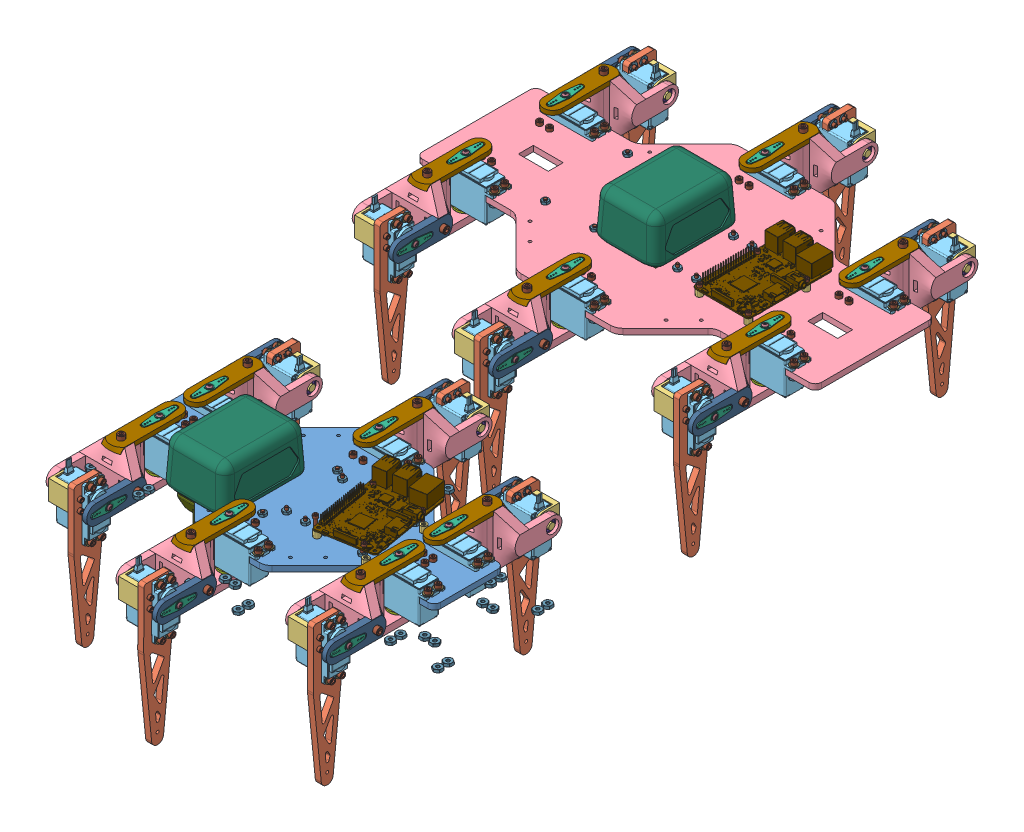
SolidWorks assembly Assem1, configuration Default. Lengths in mm. (continued)
Components (placement in the parent): (continued)
- Hexapod_NewBody-1: Hexapod_NewBody [Défaut] at origin size (371.2 181.88 349.28) (continued)
  - Battery-1: Battery [Défaut] at (-209.6397 14.6626 -46.247) x (-1 0 0) z (0 0 1) size (64.47 74.3 85.78) (continued)
    - MAKITA 4.0AH MOBILE-1: MAKITA 4.0AH MOBILE [Défaut] at (0.5853 -39.3124 91.7936) size (45.84 26.68 66.29)
  - arduinoMega-1: arduinoMega [Detailed] at (-189.11 -7.6 22.62) x (0 0 -1) z (-1 0 0) size (108.32 14.5 53.3)
  - raspberryPi3B-1: raspberryPi3B [Detailed] at (-100.6704 6.35 5.1405) x (-0.167042 0 -0.98595) z (0 1 0) size (87.05 58.5 19.5)
  - 12Channel PWM-1: 12Channel PWM [Default] at (-145.6 -5.6 15) x (-1 0 0) z (0 0 1) size (25.4 7.55 66.7)
  - DROK_090483.stp-1: DROK_090483.stp [Default] at (-77.5 -5.6 45) x (-1 0 0) z (0 -1 0) size (50.02 60 18.9)
  - socket head cap screw_ai-2: socket head cap screw_ai [HX-SHCS 0.138-32x0.625x0.625-N] at (-40.288 3.5052 19.09) x (0 -1 0) z (1 0 0) size (19.38 5.74 5.74)
  - socket head cap screw_ai-3: socket head cap screw_ai [HX-SHCS 0.138-32x0.625x0.625-N] at (-50.288 3.5052 19.09) x (0 -1 0) z (0.5 0 0.866025) size (19.38 5.74 5.74)
  - socket head cap screw_ai-4: socket head cap screw_ai [HX-SHCS 0.138-32x0.625x0.625-N] at (-50.288 3.5052 10.91) x (0 -1 0) z (1 0 0) size (19.38 5.74 5.74)
  - socket head cap screw_ai-5: socket head cap screw_ai [HX-SHCS 0.138-32x0.625x0.625-N] at (-40.288 3.5052 10.91) x (0 -1 0) z (1 0 0) size (19.38 5.74 5.74)
  - socket head cap screw_ai-6: socket head cap screw_ai [HX-SHCS 0.138-32x0.625x0.625-N] at (-170.288 3.5052 69.09) x (0 -1 0) z (1 0 0) size (19.38 5.74 5.74)
  - socket head cap screw_ai-7: socket head cap screw_ai [HX-SHCS 0.138-32x0.625x0.625-N] at (-160.288 3.5052 69.09) x (0 -1 0) z (1 0 0) size (19.38 5.74 5.74)
  - socket head cap screw_ai-14: socket head cap screw_ai [HX-SHCS 0.138-32x0.625x0.625-N] at (-160.288 3.5052 -39.09) x (0 -1 0) z (1 0 0) size (19.38 5.74 5.74)
  - socket head cap screw_ai-15: socket head cap screw_ai [HX-SHCS 0.138-32x0.625x0.625-N] at (-170.288 3.5052 -39.09) x (0 -1 0) z (1 0 0) size (19.38 5.74 5.74)
  - socket head cap screw_ai-16: socket head cap screw_ai [HX-SHCS 0.138-32x0.625x0.625-N] at (-280.288 3.5052 19.09) x (0 -1 0) z (1 0 0) size (19.38 5.74 5.74)
  - socket head cap screw_ai-17: socket head cap screw_ai [HX-SHCS 0.138-32x0.625x0.625-N] at (-290.288 3.5052 19.09) x (0 -1 0) z (0.5 0 0.866025) size (19.38 5.74 5.74)
  - socket head cap screw_ai-18: socket head cap screw_ai [HX-SHCS 0.138-32x0.625x0.625-N] at (-290.288 3.5052 10.91) x (0 -1 0) z (1 0 0) size (19.38 5.74 5.74)
  - socket head cap screw_ai-19: socket head cap screw_ai [HX-SHCS 0.138-32x0.625x0.625-N] at (-280.288 3.5052 10.91) x (0 -1 0) z (1 0 0) size (19.38 5.74 5.74)
  - machine screw nut hex_ai-60: machine screw nut hex_ai [MSHXNUT 0.138-32-D-N] at (-298.75 -8.4956 -15.08) x (1 0 0) z (0 -1 0) size (7.92 9.15 2.9)
  - machine screw nut hex_ai-65: machine screw nut hex_ai [MSHXNUT 0.138-32-D-N] at (-298.75 -8.4956 -4.92) x (1 0 0) z (0 -1 0) size (7.92 9.15 2.9)
  - machine screw nut hex_ai-70: machine screw nut hex_ai [MSHXNUT 0.138-32-D-N] at (-251.252 -8.4956 -4.92) x (0.5 0 0.866025) z (0 -1 0) size (7.92 9.15 2.9)
  - machine screw nut hex_ai-75: machine screw nut hex_ai [MSHXNUT 0.138-32-D-N] at (-251.252 -8.4956 -15.08) x (0.5 0 0.866025) z (0 -1 0) size (7.92 9.15 2.9)
  - machine screw nut hex_ai-80: machine screw nut hex_ai [MSHXNUT 0.138-32-D-N] at (-280.288 -13.5656 10.91) x (0 0 1) z (0 -1 0) size (7.92 9.15 2.9)
  - machine screw nut hex_ai-85: machine screw nut hex_ai [MSHXNUT 0.138-32-D-N] at (-290.288 -13.5656 10.91) x (0 0 1) z (0 -1 0) size (7.92 9.15 2.9)
  - machine screw nut hex_ai-63: machine screw nut hex_ai [MSHXNUT 0.138-32-D-N] at (-148.75 -8.4956 -65.08) x (1 0 0) z (0 -1 0) size (7.92 9.15 2.9)
  - machine screw nut hex_ai-68: machine screw nut hex_ai [MSHXNUT 0.138-32-D-N] at (-148.75 -8.4956 -54.92) x (1 0 0) z (0 -1 0) size (7.92 9.15 2.9)
  - machine screw nut hex_ai-73: machine screw nut hex_ai [MSHXNUT 0.138-32-D-N] at (-101.252 -8.4956 -54.92) x (0.5 0 0.866025) z (0 -1 0) size (7.92 9.15 2.9)
  - machine screw nut hex_ai-78: machine screw nut hex_ai [MSHXNUT 0.138-32-D-N] at (-101.252 -8.4956 -65.08) x (0.5 0 0.866025) z (0 -1 0) size (7.92 9.15 2.9)
  - machine screw nut hex_ai-83: machine screw nut hex_ai [MSHXNUT 0.138-32-D-N] at (-130.288 -13.5656 -39.09) x (0 0 1) z (0 -1 0) size (7.92 9.15 2.9)
  - machine screw nut hex_ai-86: machine screw nut hex_ai [MSHXNUT 0.138-32-D-N] at (-140.288 -13.5656 -39.09) x (0 0 1) z (0 -1 0) size (7.92 9.15 2.9)
  - machine screw nut hex_ai-87: machine screw nut hex_ai [MSHXNUT 0.138-32-D-N] at (9.712 -13.5656 10.91) x (0 0 1) z (0 -1 0) size (7.92 9.15 2.9)
  - machine screw nut hex_ai-84: machine screw nut hex_ai [MSHXNUT 0.138-32-D-N] at (19.712 -13.5656 10.91) x (0 0 1) z (0 -1 0) size (7.92 9.15 2.9)
  - machine screw nut hex_ai-74: machine screw nut hex_ai [MSHXNUT 0.138-32-D-N] at (48.748 -8.4956 -4.92) x (0.5 0 0.866025) z (0 -1 0) size (7.92 9.15 2.9)
  - machine screw nut hex_ai-79: machine screw nut hex_ai [MSHXNUT 0.138-32-D-N] at (48.748 -8.4956 -15.08) x (0.5 0 0.866025) z (0 -1 0) size (7.92 9.15 2.9)
  - machine screw nut hex_ai-69: machine screw nut hex_ai [MSHXNUT 0.138-32-D-N] at (1.25 -8.4956 -4.92) x (1 0 0) z (0 -1 0) size (7.92 9.15 2.9)
  - machine screw nut hex_ai-64: machine screw nut hex_ai [MSHXNUT 0.138-32-D-N] at (1.25 -8.4956 -15.08) x (1 0 0) z (0 -1 0) size (7.92 9.15 2.9)
  - machine screw nut hex_ai-88: machine screw nut hex_ai [MSHXNUT 0.138-32-D-N] at (-290.288 -10.67 69.09) x (0 0 -1) z (0 1 0) size (7.92 9.15 2.9)
  - machine screw nut hex_ai-89: machine screw nut hex_ai [MSHXNUT 0.138-32-D-N] at (-280.288 -10.67 69.09) x (0 0 -1) z (0 1 0) size (7.92 9.15 2.9)
  - machine screw nut hex_ai-90: machine screw nut hex_ai [MSHXNUT 0.138-32-D-N] at (-251.252 -5.6 84.92) x (0.5 0 -0.866025) z (0 1 0) size (7.92 9.15 2.9)
  - machine screw nut hex_ai-91: machine screw nut hex_ai [MSHXNUT 0.138-32-D-N] at (-251.252 -5.6 95.08) x (0.5 0 -0.866025) z (0 1 0) size (7.92 9.15 2.9)
  - machine screw nut hex_ai-92: machine screw nut hex_ai [MSHXNUT 0.138-32-D-N] at (-298.75 -5.6 84.92) x (1 0 0) z (0 1 0) size (7.92 9.15 2.9)
  - machine screw nut hex_ai-93: machine screw nut hex_ai [MSHXNUT 0.138-32-D-N] at (-298.75 -5.6 95.08) x (1 0 0) z (0 1 0) size (7.92 9.15 2.9)
  - machine screw nut hex_ai-94: machine screw nut hex_ai [MSHXNUT 0.138-32-D-N] at (-148.75 -5.6 145.08) x (1 0 0) z (0 1 0) size (7.92 9.15 2.9)
  - machine screw nut hex_ai-95: machine screw nut hex_ai [MSHXNUT 0.138-32-D-N] at (-148.75 -5.6 134.92) x (1 0 0) z (0 1 0) size (7.92 9.15 2.9)
  - machine screw nut hex_ai-96: machine screw nut hex_ai [MSHXNUT 0.138-32-D-N] at (-101.252 -5.6 134.92) x (0.5 0 -0.866025) z (0 1 0) size (7.92 9.15 2.9)
  - machine screw nut hex_ai-97: machine screw nut hex_ai [MSHXNUT 0.138-32-D-N] at (-101.252 -5.6 145.08) x (0.5 0 -0.866025) z (0 1 0) size (7.92 9.15 2.9)
  - machine screw nut hex_ai-98: machine screw nut hex_ai [MSHXNUT 0.138-32-D-N] at (-130.288 -10.67 119.09) x (0 0 -1) z (0 1 0) size (7.92 9.15 2.9)
  - machine screw nut hex_ai-99: machine screw nut hex_ai [MSHXNUT 0.138-32-D-N] at (-140.288 -10.67 119.09) x (0 0 -1) z (0 1 0) size (7.92 9.15 2.9)
  - machine screw nut hex_ai-100: machine screw nut hex_ai [MSHXNUT 0.138-32-D-N] at (9.712 -10.67 69.09) x (0 0 -1) z (0 1 0) size (7.92 9.15 2.9)
  - machine screw nut hex_ai-101: machine screw nut hex_ai [MSHXNUT 0.138-32-D-N] at (19.712 -10.67 69.09) x (0 0 -1) z (0 1 0) size (7.92 9.15 2.9)
  - machine screw nut hex_ai-102: machine screw nut hex_ai [MSHXNUT 0.138-32-D-N] at (48.748 -5.6 84.92) x (0.5 0 -0.866025) z (0 1 0) size (7.92 9.15 2.9)
  - machine screw nut hex_ai-103: machine screw nut hex_ai [MSHXNUT 0.138-32-D-N] at (48.748 -5.6 95.08) x (0.5 0 -0.866025) z (0 1 0) size (7.92 9.15 2.9)
  - machine screw nut hex_ai-104: machine screw nut hex_ai [MSHXNUT 0.138-32-D-N] at (1.25 -5.6 84.92) x (1 0 0) z (0 1 0) size (7.92 9.15 2.9)
  - machine screw nut hex_ai-105: machine screw nut hex_ai [MSHXNUT 0.138-32-D-N] at (1.25 -5.6 95.08) x (1 0 0) z (0 1 0) size (7.92 9.15 2.9)
  - socket head cap screw_ai-20: socket head cap screw_ai [HX-SHCS 0.138-32x0.5x0.5-N] at (-165 -12.6052 56.88) x (0 1 0) z (-0.5 0 -0.866025) size (16.21 5.74 5.74)
  - socket head cap screw_ai-21: socket head cap screw_ai [HX-SHCS 0.138-32x0.5x0.5-N] at (-213.22 -12.6052 -24.36) x (0 1 0) z (1 0 0) size (16.21 5.74 5.74)
  - socket head cap screw_ai-22: socket head cap screw_ai [HX-SHCS 0.138-32x0.5x0.5-N] at (-165 -12.6052 -18) x (0 1 0) z (-0.5 0 -0.866025) size (16.21 5.74 5.74)
  - socket head cap screw_ai-23: socket head cap screw_ai [HX-SHCS 0.138-32x0.5x0.5-N] at (-213.22 -12.6052 58.11) x (0 1 0) z (-1 0 0) size (16.21 5.74 5.74)
  - machine screw nut hex_ai-106: machine screw nut hex_ai [MSHXNUT 0.112-40-D-N] at (-213.22 2.4892 -24.36) x (1 0 0) z (0 1 0) size (6.35 7.33 2.49)
  - machine screw nut hex_ai-107: machine screw nut hex_ai [MSHXNUT 0.112-40-D-N] at (-213.22 2.4892 58.11) x (1 0 0) z (0 1 0) size (6.35 7.33 2.49)
  - machine screw nut hex_ai-108: machine screw nut hex_ai [MSHXNUT 0.112-40-D-N] at (-165 2.4892 -18) x (1 0 0) z (0 1 0) size (6.35 7.33 2.49)
  - machine screw nut hex_ai-109: machine screw nut hex_ai [MSHXNUT 0.112-40-D-N] at (-165 2.4892 56.88) x (1 0 0) z (0 1 0) size (6.35 7.33 2.49)
  - socket head cap screw_ai-24: socket head cap screw_ai [HX-SHCS 0.138-32x0.5x0.5-N] at (-117.315 -10.3052 -11.415) x (0 1 0) z (-0.5 0 -0.866025) size (16.21 5.74 5.74)
  - machine screw nut hex_ai-110: machine screw nut hex_ai [MSHXNUT 0.112-40-D-N] at (-117.315 2.4892 -11.415) x (1 0 0) z (0 1 0) size (6.35 7.33 2.49)
  - socket head cap screw_ai-25: socket head cap screw_ai [HX-SHCS 0.138-32x0.5x0.5-N] at (-80.685 -10.3052 -11.415) x (0 1 0) z (-0.5 0 -0.866025) size (16.21 5.74 5.74)
  - socket head cap screw_ai-26: socket head cap screw_ai [HX-SHCS 0.138-32x0.5x0.5-N] at (-117.315 -10.3052 41.415) x (0 1 0) z (-0.5 0 -0.866025) size (16.21 5.74 5.74)
  - socket head cap screw_ai-27: socket head cap screw_ai [HX-SHCS 0.138-32x0.5x0.5-N] at (-80.685 -10.3052 41.415) x (0 1 0) z (-0.5 0 -0.866025) size (16.21 5.74 5.74)
  - machine screw nut hex_ai-111: machine screw nut hex_ai [MSHXNUT 0.112-40-D-N] at (-80.685 2.4892 -11.415) x (1 0 0) z (0 1 0) size (6.35 7.33 2.49)
  - machine screw nut hex_ai-112: machine screw nut hex_ai [MSHXNUT 0.112-40-D-N] at (-117.315 2.4892 41.415) x (1 0 0) z (0 1 0) size (6.35 7.33 2.49)
  - machine screw nut hex_ai-113: machine screw nut hex_ai [MSHXNUT 0.112-40-D-N] at (-80.685 2.4892 41.415) x (1 0 0) z (0 1 0) size (6.35 7.33 2.49)
  - 1_4_Round_Aluminum_Standoff.step-1: 1_4_Round_Aluminum_Standoff.step [Défaut] at (-70 0 -9.5) x (0.963282 0 -0.268492) z (0.268492 0 0.963282) size (6.34 6.36 6.34)
  - socket head cap screw_ai-28: socket head cap screw_ai [HX-SHCS 0.112-40x1x0.75-N] at (-79.6885 10.4948 -17.6851) x (0 -1 0) z (0.637638 0 0.770336) size (28.24 4.65 4.65)
  - machine screw nut hex_ai-114: machine screw nut hex_ai [MSHXNUT 0.112-40-D-N] at (-79.6885 -8.0892 -17.6851) x (1 0 0) z (0 -1 0) size (6.35 7.33 2.49)
  - 1_4_Round_Aluminum_Standoff.step-2: 1_4_Round_Aluminum_Standoff.step [Défaut] at (-119 0 -9.5) x (0.963282 0 -0.268492) z (0.268492 0 0.963282) size (6.34 6.36 6.34)
  - 1_4_Round_Aluminum_Standoff.step-3: 1_4_Round_Aluminum_Standoff.step [Défaut] at (-70 0 48.5) x (0.963282 0 -0.268492) z (0.268492 0 0.963282) size (6.34 6.36 6.34)
  - 1_4_Round_Aluminum_Standoff.step-4: 1_4_Round_Aluminum_Standoff.step [Défaut] at (-119 0 48.5) x (0.963282 0 -0.268492) z (0.268492 0 0.963282) size (6.34 6.36 6.34)
  - machine screw nut hex_ai-115: machine screw nut hex_ai [MSHXNUT 0.112-40-D-N] at (-128.6885 -8.0892 -17.6851) x (1 0 0) z (0 -1 0) size (6.35 7.33 2.49)
  - machine screw nut hex_ai-116: machine screw nut hex_ai [MSHXNUT 0.112-40-D-N] at (-79.6885 -8.0892 40.3149) x (1 0 0) z (0 -1 0) size (6.35 7.33 2.49)
  - machine screw nut hex_ai-117: machine screw nut hex_ai [MSHXNUT 0.112-40-D-N] at (-128.6885 -8.0892 40.3149) x (1 0 0) z (0 -1 0) size (6.35 7.33 2.49)
  - socket head cap screw_ai-29: socket head cap screw_ai [HX-SHCS 0.112-40x1x0.75-N] at (-128.6885 10.4948 -17.6851) x (0 -1 0) z (0.637638 0 0.770336) size (28.24 4.65 4.65)
  - socket head cap screw_ai-30: socket head cap screw_ai [HX-SHCS 0.112-40x1x0.75-N] at (-79.6885 10.4948 40.3149) x (0 -1 0) z (0.637638 0 0.770336) size (28.24 4.65 4.65)
  - socket head cap screw_ai-31: socket head cap screw_ai [HX-SHCS 0.112-40x1x0.75-N] at (-128.6885 10.4948 40.3149) x (0 -1 0) z (0.637638 0 0.770336) size (28.24 4.65 4.65)
  - socket head cap screw_ai-32: socket head cap screw_ai [HX-SHCS 0.112-40x0.5x0.5-N] at (-155 -9.9448 -12.95) x (0 1 0) z (-1 0 0) size (15.54 4.65 4.65)
  - machine screw nut hex_ai-118: machine screw nut hex_ai [MSHXNUT 0.112-40-D-N] at (-155 2.4892 -12.95) x (1 0 0) z (0 1 0) size (6.35 7.33 2.49)
  - socket head cap screw_ai-33: socket head cap screw_ai [HX-SHCS 0.112-40x0.5x0.5-N] at (-136.2 -9.9448 -12.95) x (0 1 0) z (-1 0 0) size (15.54 4.65 4.65)
  - socket head cap screw_ai-34: socket head cap screw_ai [HX-SHCS 0.112-40x0.5x0.5-N] at (-155 -9.9448 42.95) x (0 1 0) z (-1 0 0) size (15.54 4.65 4.65)
  - socket head cap screw_ai-35: socket head cap screw_ai [HX-SHCS 0.112-40x0.5x0.5-N] at (-136.2 -9.9448 42.95) x (0 1 0) z (-1 0 0) size (15.54 4.65 4.65)
  - machine screw nut hex_ai-119: machine screw nut hex_ai [MSHXNUT 0.112-40-D-N] at (-136.2 2.4892 -12.95) x (1 0 0) z (0 1 0) size (6.35 7.33 2.49)
  - machine screw nut hex_ai-120: machine screw nut hex_ai [MSHXNUT 0.112-40-D-N] at (-155 2.4892 42.95) x (1 0 0) z (0 1 0) size (6.35 7.33 2.49)
  - machine screw nut hex_ai-121: machine screw nut hex_ai [MSHXNUT 0.112-40-D-N] at (-136.2 2.4892 42.95) x (1 0 0) z (0 1 0) size (6.35 7.33 2.49)
- Hexapod-1: Hexapod [Défaut] at (0 0 -431.8) size (400 181.88 399.28)
  - Body-5: Body [Default] at (-400 -5.6 40) x (1 0 0) z (0 1 0) size (400 220 5.6)
  - Leg-6: Leg [Default] at (-69.94 -26.67 -0.094) size (70.67 158.62 124.58)
    - Foot_V2_Straight-1: Foot_V2_Straight [Default] at (5.4563 4.661 -91.3712) x (0.005731 -0.001458 0.999983) z (-0.999984 0 0.005731) size (28 145.4 6)
    - bearing_mount_foot-1: bearing_mount_foot [Default] at (5.5782 16.6093 -99.7646) x (-0.005731 0.001458 -0.999983) z (0.999984 0 -0.005731) size (25 20 29.5)
    - Joint-1: Joint [Défaut] at (36.1468 26.4662 -54.5086) x (-0.005731 0 -0.999984) z (0 1 0) size (96.52 53.26 53.26)
    - hs-422-2: hs-422 [Défaut] at (5.505 6.6398 -77.4623) x (-0.005731 0.001458 -0.999983) z (0.000008 0.999999 0.001458) size (19.81 42.09 58.23)
    - hs-422-3: hs-422 [Défaut] at (19.939 20.701 -19.812) x (0 0 1) z (-1 0 0) size (19.81 42.09 58.23)
    - hs-422_horn_straight-1: hs-422_horn_straight [Default] at (-16.4246 16.9412 -87.2278) x (0.005731 0 0.999984) z (0 1 0) size (33.93 4.93 8.79)
    - hs-422_horn_straight-2: hs-422_horn_straight [Default] at (9.652 42.5743 -9.906) x (-0.005731 0 -0.999984) z (-0.999984 0 0.005731) size (33.93 4.93 8.79)
    - Bearing_mount_leg-1: Bearing_mount_leg [Default] at (9.652 21 2.594) x (0 0 1) z (0 -1 0) size (35 20 30)
    - Bearing-1: Bearing [Default] at (9.652 -6.7498 -9.906) x (0.84763 0 0.530588) z (-0.530588 0 0.84763) size (13.87 4.75 13.87)
    - Bearing-2: Bearing [Default] at (32.8986 16.9412 -87.5105) x (0.003061 -0.845349 0.534206) z (-0.004844 -0.534214 -0.845335) size (13.87 4.75 13.87)
    - Joint_attachment_leg-1: Joint_attachment_leg [Défaut] at (36.1468 26.4662 -54.5086) x (-0.005731 0 -0.999984) z (0 1 0) size (74.32 19.07 4.32)
    - Joint_attachment_foot-1: Joint_attachment_foot [Défaut] at (36.1468 26.4662 -54.5086) x (-0.005731 0 -0.999984) z (0 1 0) size (64.08 6.7 19.07)
    - socket_1_2_6-32_with_washer-1: socket_1_2_6-32_with_washer [Défaut] at (43.8172 -14.6702 -93.6435) x (0.999984 0 -0.005731) z (0.004959 -0.501262 0.865281) size (16.21 7.92 7.92)
      - socket head cap screw_ai-1: socket head cap screw_ai [HX-SHCS 0.138-32x0.5x0.5-N] at (-51.206 -1.62 2.0257) size (16.21 5.74 5.74)
      - flat washer type b narrow_ai-1: flat washer type b narrow_ai [Narrow FW 0.138] at (-46.888 -1.62 2.0257) size (0.81 7.92 7.92)
    - socket_1_2_6-32_with_washer-2: socket_1_2_6-32_with_washer [Défaut] at (43.8716 -19.1255 -84.1659) x (0.999984 0 -0.005731) z (0.000008 0.999999 0.001458) size (16.21 7.92 7.92)
      - socket head cap screw_ai-1: socket head cap screw_ai [HX-SHCS 0.138-32x0.5x0.5-N] at (-51.206 -1.62 2.0257) size (16.21 5.74 5.74)
      - flat washer type b narrow_ai-1: flat washer type b narrow_ai [Narrow FW 0.138] at (-46.888 -1.62 2.0257) size (0.81 7.92 7.92)
    - socket_1_2_6-32_with_washer-3: socket_1_2_6-32_with_washer [Défaut] at (43.8284 27.9935 -91.6928) x (0.999984 0 -0.005731) z (-0.004959 0.501262 -0.865281) size (16.21 7.92 7.92)
      - socket head cap screw_ai-1: socket head cap screw_ai [HX-SHCS 0.138-32x0.5x0.5-N] at (-51.206 -1.62 2.0257) size (16.21 5.74 5.74)
      - flat washer type b narrow_ai-1: flat washer type b narrow_ai [Narrow FW 0.138] at (-46.888 -1.62 2.0257) size (0.81 7.92 7.92)
    - socket_1_2_6-32_with_washer-4: socket_1_2_6-32_with_washer [Défaut] at (43.8866 27.9806 -81.533) x (0.999984 0 -0.005731) z (-0.004959 0.501262 -0.865281) size (16.21 7.92 7.92)
      - socket head cap screw_ai-1: socket head cap screw_ai [HX-SHCS 0.138-32x0.5x0.5-N] at (-51.206 -1.62 2.0257) size (16.21 5.74 5.74)
      - flat washer type b narrow_ai-1: flat washer type b narrow_ai [Narrow FW 0.138] at (-46.888 -1.62 2.0257) size (0.81 7.92 7.92)
    - socket button head cap screw_ai-2: socket button head cap screw_ai [SBHCSCREW 0.112-40x0.25-HX-N] at (-19.4218 16.9412 -87.2107) x (0.999984 0 -0.005731) z (-0.002865 0.866025 -0.499992) size (7.85 5.41 5.41)
    - socket button head cap screw_ai-3: socket button head cap screw_ai [SBHCSCREW 0.112-40x0.25-HX-N] at (9.652 45.5715 -9.906) x (0 -1 0) z (0.868877 0 0.495029) size (7.85 5.41 5.41)
    - machine screw nut hex_ai-7: machine screw nut hex_ai [MSHXNUT 0.138-32-D-N] at (5.4499 -17.0874 -92.4829) x (-0.004959 0.501262 -0.865281) z (0.999984 0 -0.005731) size (7.92 9.15 2.9)
    - machine screw nut hex_ai-8: machine screw nut hex_ai [MSHXNUT 0.138-32-D-N] at (5.5081 -17.1022 -82.3231) x (-0.004959 0.501262 -0.865281) z (-0.999984 0 0.005731) size (7.92 9.15 2.9)
    - machine screw nut hex_ai-9: machine screw nut hex_ai [MSHXNUT 0.138-32-D-N] at (5.4503 30.4106 -92.4136) x (0.000008 0.999999 0.001458) z (0.999984 0 -0.005731) size (7.92 9.15 2.9)
    - machine screw nut hex_ai-10: machine screw nut hex_ai [MSHXNUT 0.138-32-D-N] at (5.5085 30.3978 -82.2538) x (0.000008 0.999999 0.001458) z (0.999984 0 -0.005731) size (7.92 9.15 2.9)
    - socket head cap screw_ai-1: socket head cap screw_ai [HX-SHCS 0.164-32x0.5x0.5-N] at (9.4314 47.8568 -48.4033) x (0 -1 0) z (0.005731 0 0.999984) size (16.87 6.86 6.86)
    - socket head cap screw_ai-2: socket head cap screw_ai [HX-SHCS 0.164-32x0.5x0.5-N] at (-21.5482 16.9412 -59.4711) x (0.999984 0 -0.005731) z (0.005731 0 0.999984) size (16.87 6.86 6.86)
    - machine screw nut hex_ai-11: machine screw nut hex_ai [MSHXNUT 0.164-32-D-N] at (9.4314 33.127 -48.4033) x (0.868877 0 0.495029) z (0 1 0) size (8.74 10.09 3.3)
    - machine screw nut hex_ai-12: machine screw nut hex_ai [MSHXNUT 0.164-32-D-N] at (-6.8186 16.9412 -59.5556) x (0.005731 0 0.999984) z (-0.999984 0 0.005731) size (8.74 10.09 3.3)
    - socket head cap screw_ai-3: socket head cap screw_ai [HX-SHCS 0.112-40x0.5x0.5-N] at (-3.4365 11.6733 -99.7202) x (0.999984 0 -0.005731) z (0.005731 -0.001458 0.999983) size (15.54 4.65 4.65)
    - socket head cap screw_ai-4: socket head cap screw_ai [HX-SHCS 0.112-40x0.5x0.5-N] at (-3.4364 21.6733 -99.7056) x (0.999984 0 -0.005731) z (-0.005731 0.001458 -0.999983) size (15.54 4.65 4.65)
    - socket_1_2_6-32_with_washer-5: socket_1_2_6-32_with_washer [Défaut] at (-3.4199 -17.7034 -7.3903) x (0 -1 0) z (0.5 0 0.866025) size (16.21 7.92 7.92)
      - socket head cap screw_ai-1: socket head cap screw_ai [HX-SHCS 0.138-32x0.5x0.5-N] at (-51.206 -1.62 2.0257) size (16.21 5.74 5.74)
      - flat washer type b narrow_ai-1: flat washer type b narrow_ai [Narrow FW 0.138] at (-46.888 -1.62 2.0257) size (0.81 7.92 7.92)
    - socket_1_2_6-32_with_washer-6: socket_1_2_6-32_with_washer [Défaut] at (44.0781 -17.7034 -17.5503) x (0 -1 0) z (0.5 0 0.866025) size (16.21 7.92 7.92)
      - socket head cap screw_ai-1: socket head cap screw_ai [HX-SHCS 0.138-32x0.5x0.5-N] at (-51.206 -1.62 2.0257) size (16.21 5.74 5.74)
      - flat washer type b narrow_ai-1: flat washer type b narrow_ai [Narrow FW 0.138] at (-46.888 -1.62 2.0257) size (0.81 7.92 7.92)
    - socket_1_2_6-32_with_washer-7: socket_1_2_6-32_with_washer [Défaut] at (-3.4199 -17.7034 -17.5503) x (0 -1 0) z (0.5 0 0.866025) size (16.21 7.92 7.92)
      - socket head cap screw_ai-1: socket head cap screw_ai [HX-SHCS 0.138-32x0.5x0.5-N] at (-51.206 -1.62 2.0257) size (16.21 5.74 5.74)
      - flat washer type b narrow_ai-1: flat washer type b narrow_ai [Narrow FW 0.138] at (-46.888 -1.62 2.0257) size (0.81 7.92 7.92)
    - socket_1_2_6-32_with_washer-8: socket_1_2_6-32_with_washer [Défaut] at (44.0781 -17.7034 -7.3903) x (0 -1 0) z (0.5 0 0.866025) size (16.21 7.92 7.92)
      - socket head cap screw_ai-1: socket head cap screw_ai [HX-SHCS 0.138-32x0.5x0.5-N] at (-51.206 -1.62 2.0257) size (16.21 5.74 5.74)
      - flat washer type b narrow_ai-1: flat washer type b narrow_ai [Narrow FW 0.138] at (-46.888 -1.62 2.0257) size (0.81 7.92 7.92)
  - Leg-7: Leg [Default] at (-369.94 -26.67 -0.094) size (70.67 158.62 124.58)
    - Foot_V2_Straight-1: Foot_V2_Straight [Default] at (5.4563 4.661 -91.3712) x (0.005731 -0.001458 0.999983) z (-0.999984 0 0.005731) size (28 145.4 6)
    - bearing_mount_foot-1: bearing_mount_foot [Default] at (5.5782 16.6093 -99.7646) x (-0.005731 0.001458 -0.999983) z (0.999984 0 -0.005731) size (25 20 29.5)
    - Joint-1: Joint [Défaut] at (36.1468 26.4662 -54.5086) x (-0.005731 0 -0.999984) z (0 1 0) size (96.52 53.26 53.26)
    - hs-422-2: hs-422 [Défaut] at (5.505 6.6398 -77.4623) x (-0.005731 0.001458 -0.999983) z (0.000008 0.999999 0.001458) size (19.81 42.09 58.23)
    - hs-422-3: hs-422 [Défaut] at (19.939 20.701 -19.812) x (0 0 1) z (-1 0 0) size (19.81 42.09 58.23)
    - hs-422_horn_straight-1: hs-422_horn_straight [Default] at (-16.4246 16.9412 -87.2278) x (0.005731 0 0.999984) z (0 1 0) size (33.93 4.93 8.79)
    - hs-422_horn_straight-2: hs-422_horn_straight [Default] at (9.652 42.5743 -9.906) x (-0.005731 0 -0.999984) z (-0.999984 0 0.005731) size (33.93 4.93 8.79)
    - Bearing_mount_leg-1: Bearing_mount_leg [Default] at (9.652 21 2.594) x (0 0 1) z (0 -1 0) size (35 20 30)
    - Bearing-1: Bearing [Default] at (9.652 -6.7498 -9.906) x (0.84763 0 0.530588) z (-0.530588 0 0.84763) size (13.87 4.75 13.87)
    - Bearing-2: Bearing [Default] at (32.8986 16.9412 -87.5105) x (0.003061 -0.845349 0.534206) z (-0.004844 -0.534214 -0.845335) size (13.87 4.75 13.87)
    - Joint_attachment_leg-1: Joint_attachment_leg [Défaut] at (36.1468 26.4662 -54.5086) x (-0.005731 0 -0.999984) z (0 1 0) size (74.32 19.07 4.32)
    - Joint_attachment_foot-1: Joint_attachment_foot [Défaut] at (36.1468 26.4662 -54.5086) x (-0.005731 0 -0.999984) z (0 1 0) size (64.08 6.7 19.07)
    - socket_1_2_6-32_with_washer-1: socket_1_2_6-32_with_washer [Défaut] at (43.8172 -14.6702 -93.6435) x (0.999984 0 -0.005731) z (0.004959 -0.501262 0.865281) size (16.21 7.92 7.92)
      - socket head cap screw_ai-1: socket head cap screw_ai [HX-SHCS 0.138-32x0.5x0.5-N] at (-51.206 -1.62 2.0257) size (16.21 5.74 5.74)
      - flat washer type b narrow_ai-1: flat washer type b narrow_ai [Narrow FW 0.138] at (-46.888 -1.62 2.0257) size (0.81 7.92 7.92)
    - socket_1_2_6-32_with_washer-2: socket_1_2_6-32_with_washer [Défaut] at (43.8716 -19.1255 -84.1659) x (0.999984 0 -0.005731) z (0.000008 0.999999 0.001458) size (16.21 7.92 7.92)
      - socket head cap screw_ai-1: socket head cap screw_ai [HX-SHCS 0.138-32x0.5x0.5-N] at (-51.206 -1.62 2.0257) size (16.21 5.74 5.74)
      - flat washer type b narrow_ai-1: flat washer type b narrow_ai [Narrow FW 0.138] at (-46.888 -1.62 2.0257) size (0.81 7.92 7.92)
    - socket_1_2_6-32_with_washer-3: socket_1_2_6-32_with_washer [Défaut] at (43.8284 27.9935 -91.6928) x (0.999984 0 -0.005731) z (-0.004959 0.501262 -0.865281) size (16.21 7.92 7.92)
      - socket head cap screw_ai-1: socket head cap screw_ai [HX-SHCS 0.138-32x0.5x0.5-N] at (-51.206 -1.62 2.0257) size (16.21 5.74 5.74)
      - flat washer type b narrow_ai-1: flat washer type b narrow_ai [Narrow FW 0.138] at (-46.888 -1.62 2.0257) size (0.81 7.92 7.92)
    - socket_1_2_6-32_with_washer-4: socket_1_2_6-32_with_washer [Défaut] at (43.8866 27.9806 -81.533) x (0.999984 0 -0.005731) z (-0.004959 0.501262 -0.865281) size (16.21 7.92 7.92)
      - socket head cap screw_ai-1: socket head cap screw_ai [HX-SHCS 0.138-32x0.5x0.5-N] at (-51.206 -1.62 2.0257) size (16.21 5.74 5.74)
      - flat washer type b narrow_ai-1: flat washer type b narrow_ai [Narrow FW 0.138] at (-46.888 -1.62 2.0257) size (0.81 7.92 7.92)
    - socket button head cap screw_ai-2: socket button head cap screw_ai [SBHCSCREW 0.112-40x0.25-HX-N] at (-19.4218 16.9412 -87.2107) x (0.999984 0 -0.005731) z (-0.002865 0.866025 -0.499992) size (7.85 5.41 5.41)
    - socket button head cap screw_ai-3: socket button head cap screw_ai [SBHCSCREW 0.112-40x0.25-HX-N] at (9.652 45.5715 -9.906) x (0 -1 0) z (0.868877 0 0.495029) size (7.85 5.41 5.41)
    - machine screw nut hex_ai-7: machine screw nut hex_ai [MSHXNUT 0.138-32-D-N] at (5.4499 -17.0874 -92.4829) x (-0.004959 0.501262 -0.865281) z (0.999984 0 -0.005731) size (7.92 9.15 2.9)
    - machine screw nut hex_ai-8: machine screw nut hex_ai [MSHXNUT 0.138-32-D-N] at (5.5081 -17.1022 -82.3231) x (-0.004959 0.501262 -0.865281) z (-0.999984 0 0.005731) size (7.92 9.15 2.9)
    - machine screw nut hex_ai-9: machine screw nut hex_ai [MSHXNUT 0.138-32-D-N] at (5.4503 30.4106 -92.4136) x (0.000008 0.999999 0.001458) z (0.999984 0 -0.005731) size (7.92 9.15 2.9)
    - machine screw nut hex_ai-10: machine screw nut hex_ai [MSHXNUT 0.138-32-D-N] at (5.5085 30.3978 -82.2538) x (0.000008 0.999999 0.001458) z (0.999984 0 -0.005731) size (7.92 9.15 2.9)
    - socket head cap screw_ai-1: socket head cap screw_ai [HX-SHCS 0.164-32x0.5x0.5-N] at (9.4314 47.8568 -48.4033) x (0 -1 0) z (0.005731 0 0.999984) size (16.87 6.86 6.86)
    - socket head cap screw_ai-2: socket head cap screw_ai [HX-SHCS 0.164-32x0.5x0.5-N] at (-21.5482 16.9412 -59.4711) x (0.999984 0 -0.005731) z (0.005731 0 0.999984) size (16.87 6.86 6.86)
    - machine screw nut hex_ai-11: machine screw nut hex_ai [MSHXNUT 0.164-32-D-N] at (9.4314 33.127 -48.4033) x (0.868877 0 0.495029) z (0 1 0) size (8.74 10.09 3.3)
    - machine screw nut hex_ai-12: machine screw nut hex_ai [MSHXNUT 0.164-32-D-N] at (-6.8186 16.9412 -59.5556) x (0.005731 0 0.999984) z (-0.999984 0 0.005731) size (8.74 10.09 3.3)
    - socket head cap screw_ai-3: socket head cap screw_ai [HX-SHCS 0.112-40x0.5x0.5-N] at (-3.4365 11.6733 -99.7202) x (0.999984 0 -0.005731) z (0.005731 -0.001458 0.999983) size (15.54 4.65 4.65)
    - socket head cap screw_ai-4: socket head cap screw_ai [HX-SHCS 0.112-40x0.5x0.5-N] at (-3.4364 21.6733 -99.7056) x (0.999984 0 -0.005731) z (-0.005731 0.001458 -0.999983) size (15.54 4.65 4.65)
    - socket_1_2_6-32_with_washer-5: socket_1_2_6-32_with_washer [Défaut] at (-3.4199 -17.7034 -7.3903) x (0 -1 0) z (0.5 0 0.866025) size (16.21 7.92 7.92)
      - socket head cap screw_ai-1: socket head cap screw_ai [HX-SHCS 0.138-32x0.5x0.5-N] at (-51.206 -1.62 2.0257) size (16.21 5.74 5.74)
      - flat washer type b narrow_ai-1: flat washer type b narrow_ai [Narrow FW 0.138] at (-46.888 -1.62 2.0257) size (0.81 7.92 7.92)
    - socket_1_2_6-32_with_washer-6: socket_1_2_6-32_with_washer [Défaut] at (44.0781 -17.7034 -17.5503) x (0 -1 0) z (0.5 0 0.866025) size (16.21 7.92 7.92)
      - socket head cap screw_ai-1: socket head cap screw_ai [HX-SHCS 0.138-32x0.5x0.5-N] at (-51.206 -1.62 2.0257) size (16.21 5.74 5.74)
      - flat washer type b narrow_ai-1: flat washer type b narrow_ai [Narrow FW 0.138] at (-46.888 -1.62 2.0257) size (0.81 7.92 7.92)
    - socket_1_2_6-32_with_washer-7: socket_1_2_6-32_with_washer [Défaut] at (-3.4199 -17.7034 -17.5503) x (0 -1 0) z (0.5 0 0.866025) size (16.21 7.92 7.92)
      - socket head cap screw_ai-1: socket head cap screw_ai [HX-SHCS 0.138-32x0.5x0.5-N] at (-51.206 -1.62 2.0257) size (16.21 5.74 5.74)
      - flat washer type b narrow_ai-1: flat washer type b narrow_ai [Narrow FW 0.138] at (-46.888 -1.62 2.0257) size (0.81 7.92 7.92)
    - socket_1_2_6-32_with_washer-8: socket_1_2_6-32_with_washer [Défaut] at (44.0781 -17.7034 -7.3903) x (0 -1 0) z (0.5 0 0.866025) size (16.21 7.92 7.92)
      - socket head cap screw_ai-1: socket head cap screw_ai [HX-SHCS 0.138-32x0.5x0.5-N] at (-51.206 -1.62 2.0257) size (16.21 5.74 5.74)
      - flat washer type b narrow_ai-1: flat washer type b narrow_ai [Narrow FW 0.138] at (-46.888 -1.62 2.0257) size (0.81 7.92 7.92)
  - Leg-8: Leg [Default] at (-219.94 -26.67 -50.094) size (70.67 158.62 124.58)
    - Foot_V2_Straight-1: Foot_V2_Straight [Default] at (5.4563 4.661 -91.3712) x (0.005731 -0.001458 0.999983) z (-0.999984 0 0.005731) size (28 145.4 6)
    - bearing_mount_foot-1: bearing_mount_foot [Default] at (5.5782 16.6093 -99.7646) x (-0.005731 0.001458 -0.999983) z (0.999984 0 -0.005731) size (25 20 29.5)
    - Joint-1: Joint [Défaut] at (36.1468 26.4662 -54.5086) x (-0.005731 0 -0.999984) z (0 1 0) size (96.52 53.26 53.26)
    - hs-422-2: hs-422 [Défaut] at (5.505 6.6398 -77.4623) x (-0.005731 0.001458 -0.999983) z (0.000008 0.999999 0.001458) size (19.81 42.09 58.23)
    - hs-422-3: hs-422 [Défaut] at (19.939 20.701 -19.812) x (0 0 1) z (-1 0 0) size (19.81 42.09 58.23)
    - hs-422_horn_straight-1: hs-422_horn_straight [Default] at (-16.4246 16.9412 -87.2278) x (0.005731 0 0.999984) z (0 1 0) size (33.93 4.93 8.79)
    - hs-422_horn_straight-2: hs-422_horn_straight [Default] at (9.652 42.5743 -9.906) x (-0.005731 0 -0.999984) z (-0.999984 0 0.005731) size (33.93 4.93 8.79)
    - Bearing_mount_leg-1: Bearing_mount_leg [Default] at (9.652 21 2.594) x (0 0 1) z (0 -1 0) size (35 20 30)
    - Bearing-1: Bearing [Default] at (9.652 -6.7498 -9.906) x (0.84763 0 0.530588) z (-0.530588 0 0.84763) size (13.87 4.75 13.87)
    - Bearing-2: Bearing [Default] at (32.8986 16.9412 -87.5105) x (0.003061 -0.845349 0.534206) z (-0.004844 -0.534214 -0.845335) size (13.87 4.75 13.87)
    - Joint_attachment_leg-1: Joint_attachment_leg [Défaut] at (36.1468 26.4662 -54.5086) x (-0.005731 0 -0.999984) z (0 1 0) size (74.32 19.07 4.32)
    - Joint_attachment_foot-1: Joint_attachment_foot [Défaut] at (36.1468 26.4662 -54.5086) x (-0.005731 0 -0.999984) z (0 1 0) size (64.08 6.7 19.07)
    - socket_1_2_6-32_with_washer-1: socket_1_2_6-32_with_washer [Défaut] at (43.8172 -14.6702 -93.6435) x (0.999984 0 -0.005731) z (0.004959 -0.501262 0.865281) size (16.21 7.92 7.92)
      - socket head cap screw_ai-1: socket head cap screw_ai [HX-SHCS 0.138-32x0.5x0.5-N] at (-51.206 -1.62 2.0257) size (16.21 5.74 5.74)
      - flat washer type b narrow_ai-1: flat washer type b narrow_ai [Narrow FW 0.138] at (-46.888 -1.62 2.0257) size (0.81 7.92 7.92)
    - socket_1_2_6-32_with_washer-2: socket_1_2_6-32_with_washer [Défaut] at (43.8716 -19.1255 -84.1659) x (0.999984 0 -0.005731) z (0.000008 0.999999 0.001458) size (16.21 7.92 7.92)
      - socket head cap screw_ai-1: socket head cap screw_ai [HX-SHCS 0.138-32x0.5x0.5-N] at (-51.206 -1.62 2.0257) size (16.21 5.74 5.74)
      - flat washer type b narrow_ai-1: flat washer type b narrow_ai [Narrow FW 0.138] at (-46.888 -1.62 2.0257) size (0.81 7.92 7.92)
    - socket_1_2_6-32_with_washer-3: socket_1_2_6-32_with_washer [Défaut] at (43.8284 27.9935 -91.6928) x (0.999984 0 -0.005731) z (-0.004959 0.501262 -0.865281) size (16.21 7.92 7.92)
      - socket head cap screw_ai-1: socket head cap screw_ai [HX-SHCS 0.138-32x0.5x0.5-N] at (-51.206 -1.62 2.0257) size (16.21 5.74 5.74)
      - flat washer type b narrow_ai-1: flat washer type b narrow_ai [Narrow FW 0.138] at (-46.888 -1.62 2.0257) size (0.81 7.92 7.92)
    - socket_1_2_6-32_with_washer-4: socket_1_2_6-32_with_washer [Défaut] at (43.8866 27.9806 -81.533) x (0.999984 0 -0.005731) z (-0.004959 0.501262 -0.865281) size (16.21 7.92 7.92)
      - socket head cap screw_ai-1: socket head cap screw_ai [HX-SHCS 0.138-32x0.5x0.5-N] at (-51.206 -1.62 2.0257) size (16.21 5.74 5.74)
      - flat washer type b narrow_ai-1: flat washer type b narrow_ai [Narrow FW 0.138] at (-46.888 -1.62 2.0257) size (0.81 7.92 7.92)
    - socket button head cap screw_ai-2: socket button head cap screw_ai [SBHCSCREW 0.112-40x0.25-HX-N] at (-19.4218 16.9412 -87.2107) x (0.999984 0 -0.005731) z (-0.002865 0.866025 -0.499992) size (7.85 5.41 5.41)
    - socket button head cap screw_ai-3: socket button head cap screw_ai [SBHCSCREW 0.112-40x0.25-HX-N] at (9.652 45.5715 -9.906) x (0 -1 0) z (0.868877 0 0.495029) size (7.85 5.41 5.41)
    - machine screw nut hex_ai-7: machine screw nut hex_ai [MSHXNUT 0.138-32-D-N] at (5.4499 -17.0874 -92.4829) x (-0.004959 0.501262 -0.865281) z (0.999984 0 -0.005731) size (7.92 9.15 2.9)
    - machine screw nut hex_ai-8: machine screw nut hex_ai [MSHXNUT 0.138-32-D-N] at (5.5081 -17.1022 -82.3231) x (-0.004959 0.501262 -0.865281) z (-0.999984 0 0.005731) size (7.92 9.15 2.9)
    - machine screw nut hex_ai-9: machine screw nut hex_ai [MSHXNUT 0.138-32-D-N] at (5.4503 30.4106 -92.4136) x (0.000008 0.999999 0.001458) z (0.999984 0 -0.005731) size (7.92 9.15 2.9)
    - machine screw nut hex_ai-10: machine screw nut hex_ai [MSHXNUT 0.138-32-D-N] at (5.5085 30.3978 -82.2538) x (0.000008 0.999999 0.001458) z (0.999984 0 -0.005731) size (7.92 9.15 2.9)
    - socket head cap screw_ai-1: socket head cap screw_ai [HX-SHCS 0.164-32x0.5x0.5-N] at (9.4314 47.8568 -48.4033) x (0 -1 0) z (0.005731 0 0.999984) size (16.87 6.86 6.86)
    - socket head cap screw_ai-2: socket head cap screw_ai [HX-SHCS 0.164-32x0.5x0.5-N] at (-21.5482 16.9412 -59.4711) x (0.999984 0 -0.005731) z (0.005731 0 0.999984) size (16.87 6.86 6.86)
    - machine screw nut hex_ai-11: machine screw nut hex_ai [MSHXNUT 0.164-32-D-N] at (9.4314 33.127 -48.4033) x (0.868877 0 0.495029) z (0 1 0) size (8.74 10.09 3.3)
    - machine screw nut hex_ai-12: machine screw nut hex_ai [MSHXNUT 0.164-32-D-N] at (-6.8186 16.9412 -59.5556) x (0.005731 0 0.999984) z (-0.999984 0 0.005731) size (8.74 10.09 3.3)
    - socket head cap screw_ai-3: socket head cap screw_ai [HX-SHCS 0.112-40x0.5x0.5-N] at (-3.4365 11.6733 -99.7202) x (0.999984 0 -0.005731) z (0.005731 -0.001458 0.999983) size (15.54 4.65 4.65)
    - socket head cap screw_ai-4: socket head cap screw_ai [HX-SHCS 0.112-40x0.5x0.5-N] at (-3.4364 21.6733 -99.7056) x (0.999984 0 -0.005731) z (-0.005731 0.001458 -0.999983) size (15.54 4.65 4.65)
    - socket_1_2_6-32_with_washer-5: socket_1_2_6-32_with_washer [Défaut] at (-3.4199 -17.7034 -7.3903) x (0 -1 0) z (0.5 0 0.866025) size (16.21 7.92 7.92)
      - socket head cap screw_ai-1: socket head cap screw_ai [HX-SHCS 0.138-32x0.5x0.5-N] at (-51.206 -1.62 2.0257) size (16.21 5.74 5.74)
      - flat washer type b narrow_ai-1: flat washer type b narrow_ai [Narrow FW 0.138] at (-46.888 -1.62 2.0257) size (0.81 7.92 7.92)
    - socket_1_2_6-32_with_washer-6: socket_1_2_6-32_with_washer [Défaut] at (44.0781 -17.7034 -17.5503) x (0 -1 0) z (0.5 0 0.866025) size (16.21 7.92 7.92)
      - socket head cap screw_ai-1: socket head cap screw_ai [HX-SHCS 0.138-32x0.5x0.5-N] at (-51.206 -1.62 2.0257) size (16.21 5.74 5.74)
      - flat washer type b narrow_ai-1: flat washer type b narrow_ai [Narrow FW 0.138] at (-46.888 -1.62 2.0257) size (0.81 7.92 7.92)
    - socket_1_2_6-32_with_washer-7: socket_1_2_6-32_with_washer [Défaut] at (-3.4199 -17.7034 -17.5503) x (0 -1 0) z (0.5 0 0.866025) size (16.21 7.92 7.92)
      - socket head cap screw_ai-1: socket head cap screw_ai [HX-SHCS 0.138-32x0.5x0.5-N] at (-51.206 -1.62 2.0257) size (16.21 5.74 5.74)
      - flat washer type b narrow_ai-1: flat washer type b narrow_ai [Narrow FW 0.138] at (-46.888 -1.62 2.0257) size (0.81 7.92 7.92)
    - socket_1_2_6-32_with_washer-8: socket_1_2_6-32_with_washer [Défaut] at (44.0781 -17.7034 -7.3903) x (0 -1 0) z (0.5 0 0.866025) size (16.21 7.92 7.92)
      - socket head cap screw_ai-1: socket head cap screw_ai [HX-SHCS 0.138-32x0.5x0.5-N] at (-51.206 -1.62 2.0257) size (16.21 5.74 5.74)
      - flat washer type b narrow_ai-1: flat washer type b narrow_ai [Narrow FW 0.138] at (-46.888 -1.62 2.0257) size (0.81 7.92 7.92)
  - Leg_V2(Mirror)-4: Leg_V2(Mirror) [Default] at (-369.94 -26.67 80.094) x (-1 0 0) z (0 0 -1) size (66.23 158.62 124.7)
    - Foot_V2_Straight-1: Foot_V2_Straight [Default] at (-13.3652 4.661 -91.3946) x (-0.000191 -0.001458 0.999999) z (-1 0 -0.000191) size (28 145.4 6)
    - bearing_mount_foot-1: bearing_mount_foot [Default] at (-13.1936 16.6093 -99.7872) x (0.000191 0.001458 -0.999999) z (1 0 0.000191) size (25 20 29.5)
    - Joint-1: Joint [Défaut] at (17.1065 26.4662 -54.3509) x (0.000191 0 -1) z (0 1 0) size (96.52 53.26 53.26)
    - hs-422-2: hs-422 [Défaut] at (-13.3989 6.6398 -77.4857) x (0.000191 0.001458 -0.999999) z (0 0.999999 0.001458) size (19.81 42.09 58.23)
    - hs-422-3: hs-422 [Défaut] at (-19.939 20.701 0) x (0 0 -1) z (1 0 0) size (19.81 42.09 58.23)
    - hs-422_horn_straight-1: hs-422_horn_straight [Default] at (-35.2703 16.9412 -87.3809) x (-0.000191 0 1) z (0 1 0) size (33.93 4.93 8.79)
    - hs-422_horn_straight-2: hs-422_horn_straight [Default] at (-9.652 42.5743 -9.906) x (0.000191 0 -1) z (-1 0 -0.000191) size (33.93 4.93 8.79)
    - Bearing_mount_leg-1: Bearing_mount_leg [Default] at (-9.652 21 2.594) x (0 0 1) z (0 -1 0) size (35 20 30)
    - Bearing-1: Bearing [Default] at (-9.652 -6.7498 -9.906) x (0.84763 0 0.530588) z (-0.530588 0 0.84763) size (13.87 4.75 13.87)
    - Bearing-2: Bearing [Default] at (14.0538 16.9412 -87.3715) x (-0.000107 0.826531 0.562891) z (-0.000158 -0.562891 0.826531) size (13.87 4.75 13.87)
    - Joint_attachment_leg-1: Joint_attachment_leg [Défaut] at (17.1065 26.4662 -54.3509) x (0.000191 0 -1) z (0 1 0) size (74.32 19.07 4.32)
    - Joint_attachment_foot-1: Joint_attachment_foot [Défaut] at (17.1065 26.4662 -54.3509) x (0.000191 0 -1) z (0 1 0) size (64.08 6.7 19.07)
    - socket_1_2_6-32_with_washer-1: socket_1_2_6-32_with_washer [Défaut] at (25.0085 -14.6702 -93.4398) x (1 0 0.000191) z (-0.000165 -0.501262 0.865296) size (16.21 7.92 7.92)
      - socket head cap screw_ai-1: socket head cap screw_ai [HX-SHCS 0.138-32x0.5x0.5-N] at (-51.206 -1.62 2.0257) size (16.21 5.74 5.74)
      - flat washer type b narrow_ai-1: flat washer type b narrow_ai [Narrow FW 0.138] at (-46.888 -1.62 2.0257) size (0.81 7.92 7.92)
    - socket_1_2_6-32_with_washer-2: socket_1_2_6-32_with_washer [Défaut] at (25.0067 -19.1255 -83.9619) x (1 0 0.000191) z (0 0.999999 0.001458) size (16.21 7.92 7.92)
      - socket head cap screw_ai-1: socket head cap screw_ai [HX-SHCS 0.138-32x0.5x0.5-N] at (-51.206 -1.62 2.0257) size (16.21 5.74 5.74)
      - flat washer type b narrow_ai-1: flat washer type b narrow_ai [Narrow FW 0.138] at (-46.888 -1.62 2.0257) size (0.81 7.92 7.92)
    - socket_1_2_6-32_with_washer-3: socket_1_2_6-32_with_washer [Défaut] at (25.0081 27.9935 -91.489) x (1 0 0.000191) z (0.000165 0.501262 -0.865296) size (16.21 7.92 7.92)
      - socket head cap screw_ai-1: socket head cap screw_ai [HX-SHCS 0.138-32x0.5x0.5-N] at (-51.206 -1.62 2.0257) size (16.21 5.74 5.74)
      - flat washer type b narrow_ai-1: flat washer type b narrow_ai [Narrow FW 0.138] at (-46.888 -1.62 2.0257) size (0.81 7.92 7.92)
    - socket_1_2_6-32_with_washer-4: socket_1_2_6-32_with_washer [Défaut] at (25.0062 27.9806 -81.329) x (1 0 0.000191) z (0.000165 0.501262 -0.865296) size (16.21 7.92 7.92)
      - socket head cap screw_ai-1: socket head cap screw_ai [HX-SHCS 0.138-32x0.5x0.5-N] at (-51.206 -1.62 2.0257) size (16.21 5.74 5.74)
      - flat washer type b narrow_ai-1: flat washer type b narrow_ai [Narrow FW 0.138] at (-46.888 -1.62 2.0257) size (0.81 7.92 7.92)
    - socket button head cap screw_ai-2: socket button head cap screw_ai [SBHCSCREW 0.112-40x0.25-HX-N] at (-38.2675 16.9412 -87.3815) x (1 0 0.000191) z (0.000095 0.866025 -0.5) size (7.85 5.41 5.41)
    - socket button head cap screw_ai-3: socket button head cap screw_ai [SBHCSCREW 0.112-40x0.25-HX-N] at (-9.652 45.5715 -9.906) x (0 -1 0) z (0.86593 0 0.500165) size (7.85 5.41 5.41)
    - machine screw nut hex_ai-7: machine screw nut hex_ai [MSHXNUT 0.138-32-D-N] at (-13.365 -17.0874 -92.5063) x (0.000165 0.501262 -0.865296) z (1 0 0.000191) size (7.92 9.15 2.9)
    - machine screw nut hex_ai-8: machine screw nut hex_ai [MSHXNUT 0.138-32-D-N] at (-13.367 -17.1022 -82.3463) x (0.000165 0.501262 -0.865296) z (-1 0 -0.000191) size (7.92 9.15 2.9)
    - machine screw nut hex_ai-9: machine screw nut hex_ai [MSHXNUT 0.138-32-D-N] at (-13.3651 30.4106 -92.4371) x (0 0.999999 0.001458) z (1 0 0.000191) size (7.92 9.15 2.9)
    - machine screw nut hex_ai-10: machine screw nut hex_ai [MSHXNUT 0.138-32-D-N] at (-13.367 30.3978 -82.2771) x (0 0.999999 0.001458) z (1 0 0.000191) size (7.92 9.15 2.9)
    - socket head cap screw_ai-1: socket head cap screw_ai [HX-SHCS 0.164-32x0.5x0.5-N] at (-9.6447 47.8568 -48.4039) x (0 -1 0) z (-0.000191 0 1) size (16.87 6.86 6.86)
    - socket head cap screw_ai-2: socket head cap screw_ai [HX-SHCS 0.164-32x0.5x0.5-N] at (-40.5581 16.9412 -59.655) x (1 0 0.000191) z (-0.000191 0 1) size (16.87 6.86 6.86)
    - machine screw nut hex_ai-11: machine screw nut hex_ai [MSHXNUT 0.164-32-D-N] at (-9.6447 33.127 -48.4039) x (0.86593 0 0.500165) z (0 1 0) size (8.74 10.09 3.3)
    - machine screw nut hex_ai-12: machine screw nut hex_ai [MSHXNUT 0.164-32-D-N] at (-25.8283 16.9412 -59.6522) x (-0.000191 0 1) z (-1 0 -0.000191) size (8.74 10.09 3.3)
    - socket head cap screw_ai-3: socket head cap screw_ai [HX-SHCS 0.112-40x0.5x0.5-N] at (-22.2084 11.6733 -99.7961) x (1 0 0.000191) z (-0.000191 -0.001458 0.999999) size (15.54 4.65 4.65)
    - socket head cap screw_ai-4: socket head cap screw_ai [HX-SHCS 0.112-40x0.5x0.5-N] at (-22.2084 21.6733 -99.7815) x (1 0 0.000191) z (0.000191 0.001458 -0.999999) size (15.54 4.65 4.65)
    - socket_1_2_6-32_with_washer-5: socket_1_2_6-32_with_washer [Défaut] at (3.4199 -17.7034 -12.4217) x (0 -1 0) z (-0.5 0 -0.866025) size (16.21 7.92 7.92)
      - socket head cap screw_ai-1: socket head cap screw_ai [HX-SHCS 0.138-32x0.5x0.5-N] at (-51.206 -1.62 2.0257) size (16.21 5.74 5.74)
      - flat washer type b narrow_ai-1: flat washer type b narrow_ai [Narrow FW 0.138] at (-46.888 -1.62 2.0257) size (0.81 7.92 7.92)
    - socket_1_2_6-32_with_washer-6: socket_1_2_6-32_with_washer [Défaut] at (-44.0781 -17.7034 -2.2617) x (0 -1 0) z (-0.5 0 -0.866025) size (16.21 7.92 7.92)
      - socket head cap screw_ai-1: socket head cap screw_ai [HX-SHCS 0.138-32x0.5x0.5-N] at (-51.206 -1.62 2.0257) size (16.21 5.74 5.74)
      - flat washer type b narrow_ai-1: flat washer type b narrow_ai [Narrow FW 0.138] at (-46.888 -1.62 2.0257) size (0.81 7.92 7.92)
    - socket_1_2_6-32_with_washer-7: socket_1_2_6-32_with_washer [Défaut] at (3.4199 -17.7034 -2.2617) x (0 -1 0) z (-0.5 0 -0.866025) size (16.21 7.92 7.92)
      - socket head cap screw_ai-1: socket head cap screw_ai [HX-SHCS 0.138-32x0.5x0.5-N] at (-51.206 -1.62 2.0257) size (16.21 5.74 5.74)
      - flat washer type b narrow_ai-1: flat washer type b narrow_ai [Narrow FW 0.138] at (-46.888 -1.62 2.0257) size (0.81 7.92 7.92)
    - socket_1_2_6-32_with_washer-8: socket_1_2_6-32_with_washer [Défaut] at (-44.0781 -17.7034 -12.4217) x (0 -1 0) z (-0.5 0 -0.866025) size (16.21 7.92 7.92)
      - socket head cap screw_ai-1: socket head cap screw_ai [HX-SHCS 0.138-32x0.5x0.5-N] at (-51.206 -1.62 2.0257) size (16.21 5.74 5.74)
      - flat washer type b narrow_ai-1: flat washer type b narrow_ai [Narrow FW 0.138] at (-46.888 -1.62 2.0257) size (0.81 7.92 7.92)
  - Leg_V2(Mirror)-5: Leg_V2(Mirror) [Default] at (-69.94 -26.67 80.094) x (-1 0 0) z (0 0 -1) size (66.23 158.62 124.7)
    - Foot_V2_Straight-1: Foot_V2_Straight [Default] at (-13.3652 4.661 -91.3946) x (-0.000191 -0.001458 0.999999) z (-1 0 -0.000191) size (28 145.4 6)
    - bearing_mount_foot-1: bearing_mount_foot [Default] at (-13.1936 16.6093 -99.7872) x (0.000191 0.001458 -0.999999) z (1 0 0.000191) size (25 20 29.5)
    - Joint-1: Joint [Défaut] at (17.1065 26.4662 -54.3509) x (0.000191 0 -1) z (0 1 0) size (96.52 53.26 53.26)
    - hs-422-2: hs-422 [Défaut] at (-13.3989 6.6398 -77.4857) x (0.000191 0.001458 -0.999999) z (0 0.999999 0.001458) size (19.81 42.09 58.23)
    - hs-422-3: hs-422 [Défaut] at (-19.939 20.701 0) x (0 0 -1) z (1 0 0) size (19.81 42.09 58.23)
    - hs-422_horn_straight-1: hs-422_horn_straight [Default] at (-35.2703 16.9412 -87.3809) x (-0.000191 0 1) z (0 1 0) size (33.93 4.93 8.79)
    - hs-422_horn_straight-2: hs-422_horn_straight [Default] at (-9.652 42.5743 -9.906) x (0.000191 0 -1) z (-1 0 -0.000191) size (33.93 4.93 8.79)
    - Bearing_mount_leg-1: Bearing_mount_leg [Default] at (-9.652 21 2.594) x (0 0 1) z (0 -1 0) size (35 20 30)
    - Bearing-1: Bearing [Default] at (-9.652 -6.7498 -9.906) x (0.84763 0 0.530588) z (-0.530588 0 0.84763) size (13.87 4.75 13.87)
    - Bearing-2: Bearing [Default] at (14.0538 16.9412 -87.3715) x (-0.000107 0.826531 0.562891) z (-0.000158 -0.562891 0.826531) size (13.87 4.75 13.87)
    - Joint_attachment_leg-1: Joint_attachment_leg [Défaut] at (17.1065 26.4662 -54.3509) x (0.000191 0 -1) z (0 1 0) size (74.32 19.07 4.32)
